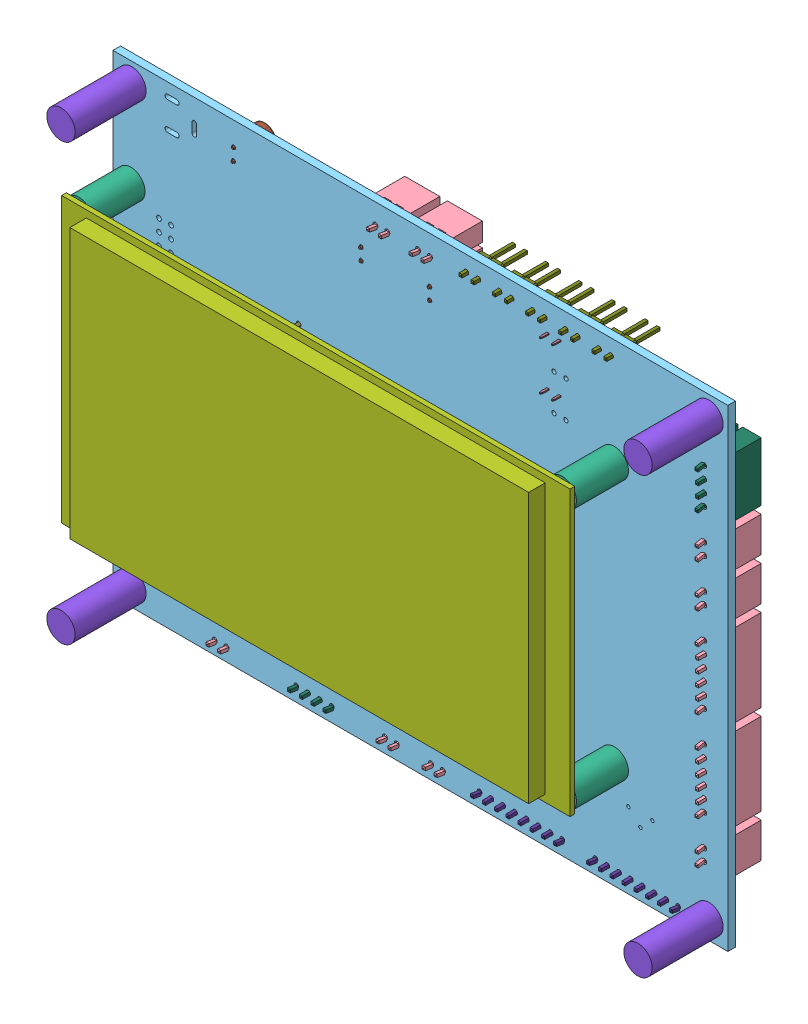
SolidWorks assembly MCU, configuration 默认. Lengths in mm.
Overall size (130 100 25.69).
427 component instances, 26 part files, 12 mates.
Components (placement in the parent):
- MCU(2)^MCU-1: MCU(2)^MCU [默认] at origin size (130 100 11.94) (virtual)
  - D_SOD-123^MCU(2)_MCU-1: D_SOD-123^MCU(2)_MCU [默认] at (95.25 63.25 -0.05) x (-1 0 0) z (0 0 -1) size (3.8 1.6 1.25) (virtual)
    - SOLID^D_SOD-123_MCU(2)_MCU-1: SOLID^D_SOD-123_MCU(2)_MCU [默认] at origin size (3.8 1.6 1.25) (virtual)
  - SOIC-8-1EP_3.9x4.9mm_P1.27mm_EP2.35x2.35mm^MCU(2)_MCU-1: SOIC-8-1EP_3.9x4.9mm_P1.27mm_EP2.35x2.35mm^MCU(2)_MCU [默认] at (12.975 8.365 -0.05) x (0 -1 0) z (0 0 -1) size (6 4.9 1.75) (virtual)
    - SOLID-0^SOIC-8-1EP_3.9x4.9mm_P1.27mm_EP2.35x2.35mm_MCU(2)_MCU-1: SOLID-0^SOIC-8-1EP_3.9x4.9mm_P1.27mm_EP2.35x2.35mm_MCU(2)_MCU [默认] at origin size (6 4.9 1.75) (virtual)
  - R_0805^MCU(2)_MCU-1: R_0805^MCU(2)_MCU [默认] at (13 3.75 -0.05) x (1 0 0) z (0 0 -1) size (2 1.25 0.5) (virtual)
    - SOLID-1^R_0805_MCU(2)_MCU-1: SOLID-1^R_0805_MCU(2)_MCU [默认] at origin size (2 1.25 0.5) (virtual)
  - R_0805^MCU(2)_MCU-2: R_0805^MCU(2)_MCU [默认] at (16.75 12 -0.05) x (0 1 0) z (0 0 -1) size (2 1.25 0.5) (virtual)
    - SOLID-1^R_0805_MCU(2)_MCU-1: SOLID-1^R_0805_MCU(2)_MCU [默认] at origin size (2 1.25 0.5) (virtual)
  - R_0805^MCU(2)_MCU-3: R_0805^MCU(2)_MCU [默认] at (8.75 12 -0.05) x (0 1 0) z (0 0 -1) size (2 1.25 0.5) (virtual)
    - SOLID-1^R_0805_MCU(2)_MCU-1: SOLID-1^R_0805_MCU(2)_MCU [默认] at origin size (2 1.25 0.5) (virtual)
  - JST_XH_B02B-XH-A_02x2.50mm_Straight^MCU(2)_MCU-1: JST_XH_B02B-XH-A_02x2.50mm_Straight^MCU(2)_MCU [默认] at (21.5 2.75 -0.05) x (1 0 0) z (0 0 -1) size (7.4 5.75 10.4) (virtual)
    - SOLID-2^JST_XH_B02B-XH-A_02x2.50mm_Straight_MCU(2)_MCU-1: SOLID-2^JST_XH_B02B-XH-A_02x2.50mm_Straight_MCU(2)_MCU [默认] at origin size (7.4 5.75 10.4) (virtual)
  - C_0805^MCU(2)_MCU-1: C_0805^MCU(2)_MCU [默认] at (12.75 13 -0.05) x (1 0 0) z (0 0 -1) size (2 1.25 0.78) (virtual)
    - SOLID-3^C_0805_MCU(2)_MCU-1: SOLID-3^C_0805_MCU(2)_MCU [默认] at origin size (2 1.25 0.78) (virtual)
  - R_0805^MCU(2)_MCU-4: R_0805^MCU(2)_MCU [默认] at (92.825 52.233 -0.05) x (1 0 0) z (0 0 -1) size (2 1.25 0.5) (virtual)
    - SOLID-1^R_0805_MCU(2)_MCU-1: SOLID-1^R_0805_MCU(2)_MCU [默认] at origin size (2 1.25 0.5) (virtual)
  - R_0805^MCU(2)_MCU-5: R_0805^MCU(2)_MCU [默认] at (92.8 50.2 -0.05) x (-1 0 0) z (0 0 -1) size (2 1.25 0.5) (virtual)
    - SOLID-1^R_0805_MCU(2)_MCU-1: SOLID-1^R_0805_MCU(2)_MCU [默认] at origin size (2 1.25 0.5) (virtual)
  - SOT-23^MCU(2)_MCU-1: SOT-23^MCU(2)_MCU [默认] at (89.35 52.05 -0.05) x (0 1 0) z (0 0 -1) size (2.5 3 1.2) (virtual)
    - SOLID-4^SOT-23_MCU(2)_MCU-1: SOLID-4^SOT-23_MCU(2)_MCU [默认] at origin size (2.5 3 1.2) (virtual)
  - D_SOD-123^MCU(2)_MCU-2: D_SOD-123^MCU(2)_MCU [默认] at (47.75 8.75 -0.05) x (1 0 0) z (0 0 -1) size (3.8 1.6 1.25) (virtual)
    - SOLID^D_SOD-123_MCU(2)_MCU-1: SOLID^D_SOD-123_MCU(2)_MCU [默认] at origin size (3.8 1.6 1.25) (virtual)
  - R_1206^MCU(2)_MCU-1: R_1206^MCU(2)_MCU [默认] at (46.8 77 -0.05) x (0 -1 0) z (0 0 -1) size (3.2 1.6 0.55) (virtual)
    - SOLID-5^R_1206_MCU(2)_MCU-1: SOLID-5^R_1206_MCU(2)_MCU [默认] at origin size (3.2 1.6 0.55) (virtual)
  - SOIC-14_3.9x8.7mm_P1.27mm^MCU(2)_MCU-1: SOIC-14_3.9x8.7mm_P1.27mm^MCU(2)_MCU [默认] at (113.4 28.8 -0.05) x (1 0 0) z (0 0 -1) size (6 8.7 1.75) (virtual)
    - SOLID-6^SOIC-14_3.9x8.7mm_P1.27mm_MCU(2)_MCU-1: SOLID-6^SOIC-14_3.9x8.7mm_P1.27mm_MCU(2)_MCU [默认] at origin size (6 8.7 1.75) (virtual)
  - R_0805^MCU(2)_MCU-6: R_0805^MCU(2)_MCU [默认] at (44 33.5 -0.05) x (0.707107 -0.707107 0) z (0 0 -1) size (2 1.25 0.5) (virtual)
    - SOLID-1^R_0805_MCU(2)_MCU-1: SOLID-1^R_0805_MCU(2)_MCU [默认] at origin size (2 1.25 0.5) (virtual)
  - C_0805^MCU(2)_MCU-2: C_0805^MCU(2)_MCU [默认] at (40.071 36.688 -0.05) x (0.707107 -0.707107 0) z (0 0 -1) size (2 1.25 0.78) (virtual)
    - SOLID-3^C_0805_MCU(2)_MCU-1: SOLID-3^C_0805_MCU(2)_MCU [默认] at origin size (2 1.25 0.78) (virtual)
  - C_0805^MCU(2)_MCU-3: C_0805^MCU(2)_MCU [默认] at (33.34 61.707 -0.05) x (-0.707107 0.707107 0) z (0 0 -1) size (2 1.25 0.78) (virtual)
    - SOLID-3^C_0805_MCU(2)_MCU-1: SOLID-3^C_0805_MCU(2)_MCU [默认] at origin size (2 1.25 0.78) (virtual)
  - C_0805^MCU(2)_MCU-4: C_0805^MCU(2)_MCU [默认] at (24.196 47.229 -0.05) x (-0.707107 -0.707107 0) z (0 0 -1) size (2 1.25 0.78) (virtual)
    - SOLID-3^C_0805_MCU(2)_MCU-1: SOLID-3^C_0805_MCU(2)_MCU [默认] at origin size (2 1.25 0.78) (virtual)
  - D_SOD-123^MCU(2)_MCU-3: D_SOD-123^MCU(2)_MCU [默认] at (70.932 14.59 -0.05) x (1 0 0) z (0 0 -1) size (3.8 1.6 1.25) (virtual)
    - SOLID^D_SOD-123_MCU(2)_MCU-1: SOLID^D_SOD-123_MCU(2)_MCU [默认] at origin size (3.8 1.6 1.25) (virtual)
  - R_0805^MCU(2)_MCU-7: R_0805^MCU(2)_MCU [默认] at (65.598 8.24 -0.05) x (-1 0 0) z (0 0 -1) size (2 1.25 0.5) (virtual)
    - SOLID-1^R_0805_MCU(2)_MCU-1: SOLID-1^R_0805_MCU(2)_MCU [默认] at origin size (2 1.25 0.5) (virtual)
  - R_0805^MCU(2)_MCU-8: R_0805^MCU(2)_MCU [默认] at (40.25 95 -0.05) x (0 -1 0) z (0 0 -1) size (2 1.25 0.5) (virtual)
    - SOLID-1^R_0805_MCU(2)_MCU-1: SOLID-1^R_0805_MCU(2)_MCU [默认] at origin size (2 1.25 0.5) (virtual)
  - R_0805^MCU(2)_MCU-9: R_0805^MCU(2)_MCU [默认] at (125.5 8.75 -0.05) x (1 0 0) z (0 0 -1) size (2 1.25 0.5) (virtual)
    - SOLID-1^R_0805_MCU(2)_MCU-1: SOLID-1^R_0805_MCU(2)_MCU [默认] at origin size (2 1.25 0.5) (virtual)
  - R_0805^MCU(2)_MCU-10: R_0805^MCU(2)_MCU [默认] at (102 34.25 -0.05) x (1 0 0) z (0 0 -1) size (2 1.25 0.5) (virtual)
    - SOLID-1^R_0805_MCU(2)_MCU-1: SOLID-1^R_0805_MCU(2)_MCU [默认] at origin size (2 1.25 0.5) (virtual)
  - R_0805^MCU(2)_MCU-11: R_0805^MCU(2)_MCU [默认] at (101.5 45.25 -0.05) x (1 0 0) z (0 0 -1) size (2 1.25 0.5) (virtual)
    - SOLID-1^R_0805_MCU(2)_MCU-1: SOLID-1^R_0805_MCU(2)_MCU [默认] at origin size (2 1.25 0.5) (virtual)
  - R_0805^MCU(2)_MCU-12: R_0805^MCU(2)_MCU [默认] at (99 73.75 -0.05) x (0 1 0) z (0 0 -1) size (2 1.25 0.5) (virtual)
    - SOLID-1^R_0805_MCU(2)_MCU-1: SOLID-1^R_0805_MCU(2)_MCU [默认] at origin size (2 1.25 0.5) (virtual)
  - R_0805^MCU(2)_MCU-13: R_0805^MCU(2)_MCU [默认] at (93.5 73.75 -0.05) x (0 1 0) z (0 0 -1) size (2 1.25 0.5) (virtual)
    - SOLID-1^R_0805_MCU(2)_MCU-1: SOLID-1^R_0805_MCU(2)_MCU [默认] at origin size (2 1.25 0.5) (virtual)
  - R_0805^MCU(2)_MCU-14: R_0805^MCU(2)_MCU [默认] at (107.5 54.75 -0.05) x (1 0 0) z (0 0 -1) size (2 1.25 0.5) (virtual)
    - SOLID-1^R_0805_MCU(2)_MCU-1: SOLID-1^R_0805_MCU(2)_MCU [默认] at origin size (2 1.25 0.5) (virtual)
  - R_0805^MCU(2)_MCU-15: R_0805^MCU(2)_MCU [默认] at (109 60.25 -0.05) x (1 0 0) z (0 0 -1) size (2 1.25 0.5) (virtual)
    - SOLID-1^R_0805_MCU(2)_MCU-1: SOLID-1^R_0805_MCU(2)_MCU [默认] at origin size (2 1.25 0.5) (virtual)
  - R_0805^MCU(2)_MCU-16: R_0805^MCU(2)_MCU [默认] at (43.25 8.45 -0.05) x (-1 0 0) z (0 0 -1) size (2 1.25 0.5) (virtual)
    - SOLID-1^R_0805_MCU(2)_MCU-1: SOLID-1^R_0805_MCU(2)_MCU [默认] at origin size (2 1.25 0.5) (virtual)
  - R_0805^MCU(2)_MCU-17: R_0805^MCU(2)_MCU [默认] at (40 8.45 -0.05) x (-1 0 0) z (0 0 -1) size (2 1.25 0.5) (virtual)
    - SOLID-1^R_0805_MCU(2)_MCU-1: SOLID-1^R_0805_MCU(2)_MCU [默认] at origin size (2 1.25 0.5) (virtual)
  - R_0805^MCU(2)_MCU-18: R_0805^MCU(2)_MCU [默认] at (83 93.5 -0.05) x (-1 0 0) z (0 0 -1) size (2 1.25 0.5) (virtual)
    - SOLID-1^R_0805_MCU(2)_MCU-1: SOLID-1^R_0805_MCU(2)_MCU [默认] at origin size (2 1.25 0.5) (virtual)
  - R_0805^MCU(2)_MCU-19: R_0805^MCU(2)_MCU [默认] at (76 93.5 -0.05) x (-1 0 0) z (0 0 -1) size (2 1.25 0.5) (virtual)
    - SOLID-1^R_0805_MCU(2)_MCU-1: SOLID-1^R_0805_MCU(2)_MCU [默认] at origin size (2 1.25 0.5) (virtual)
  - R_0805^MCU(2)_MCU-20: R_0805^MCU(2)_MCU [默认] at (90 93.5 -0.05) x (1 0 0) z (0 0 -1) size (2 1.25 0.5) (virtual)
    - SOLID-1^R_0805_MCU(2)_MCU-1: SOLID-1^R_0805_MCU(2)_MCU [默认] at origin size (2 1.25 0.5) (virtual)
  - SOIC-16_3.9x9.9mm_P1.27mm^MCU(2)_MCU-1: SOIC-16_3.9x9.9mm_P1.27mm^MCU(2)_MCU [默认] at (43.9 16.7 -0.05) x (0 -1 0) z (0 0 -1) size (6 9.9 1.75) (virtual)
    - SOLID-7^SOIC-16_3.9x9.9mm_P1.27mm_MCU(2)_MCU-1: SOLID-7^SOIC-16_3.9x9.9mm_P1.27mm_MCU(2)_MCU [默认] at origin size (6 9.9 1.75) (virtual)
  - SOT-23-5^MCU(2)_MCU-1: SOT-23-5^MCU(2)_MCU [默认] at (106.5 90 -0.05) x (-1 0 0) z (0 0 -1) size (2.8 2.9 1.55) (virtual)
    - SOLID-8^SOT-23-5_MCU(2)_MCU-1: SOLID-8^SOT-23-5_MCU(2)_MCU [默认] at origin size (2.8 2.9 1.55) (virtual)
  - R_0805^MCU(2)_MCU-21: R_0805^MCU(2)_MCU [默认] at (108.5 93.5 -0.05) x (-1 0 0) z (0 0 -1) size (2 1.25 0.5) (virtual)
    - SOLID-1^R_0805_MCU(2)_MCU-1: SOLID-1^R_0805_MCU(2)_MCU [默认] at origin size (2 1.25 0.5) (virtual)
  - C_0805^MCU(2)_MCU-5: C_0805^MCU(2)_MCU [默认] at (37.023 18.315 -0.05) x (0 1 0) z (0 0 -1) size (2 1.25 0.78) (virtual)
    - SOLID-3^C_0805_MCU(2)_MCU-1: SOLID-3^C_0805_MCU(2)_MCU [默认] at origin size (2 1.25 0.78) (virtual)
  - C_0805^MCU(2)_MCU-6: C_0805^MCU(2)_MCU [默认] at (47.765 22.2 -0.05) x (-1 0 0) z (0 0 -1) size (2 1.25 0.78) (virtual)
    - SOLID-3^C_0805_MCU(2)_MCU-1: SOLID-3^C_0805_MCU(2)_MCU [默认] at origin size (2 1.25 0.78) (virtual)
  - C_0805^MCU(2)_MCU-7: C_0805^MCU(2)_MCU [默认] at (44.015 22.2 -0.05) x (-1 0 0) z (0 0 -1) size (2 1.25 0.78) (virtual)
    - SOLID-3^C_0805_MCU(2)_MCU-1: SOLID-3^C_0805_MCU(2)_MCU [默认] at origin size (2 1.25 0.78) (virtual)
  - C_0805^MCU(2)_MCU-8: C_0805^MCU(2)_MCU [默认] at (37.15 12.812 -0.05) x (0 -1 0) z (0 0 -1) size (2 1.25 0.78) (virtual)
    - SOLID-3^C_0805_MCU(2)_MCU-1: SOLID-3^C_0805_MCU(2)_MCU [默认] at origin size (2 1.25 0.78) (virtual)
  - C_0805^MCU(2)_MCU-9: C_0805^MCU(2)_MCU [默认] at (40.265 22.2 -0.05) x (1 0 0) z (0 0 -1) size (2 1.25 0.78) (virtual)
    - SOLID-3^C_0805_MCU(2)_MCU-1: SOLID-3^C_0805_MCU(2)_MCU [默认] at origin size (2 1.25 0.78) (virtual)
  - D_SOD-123^MCU(2)_MCU-4: D_SOD-123^MCU(2)_MCU [默认] at (68.6 18.866 -0.05) x (1 0 0) z (0 0 -1) size (3.8 1.6 1.25) (virtual)
    - SOLID^D_SOD-123_MCU(2)_MCU-1: SOLID^D_SOD-123_MCU(2)_MCU [默认] at origin size (3.8 1.6 1.25) (virtual)
  - D_SOD-123^MCU(2)_MCU-5: D_SOD-123^MCU(2)_MCU [默认] at (68.6 16.866 -0.05) x (1 0 0) z (0 0 -1) size (3.8 1.6 1.25) (virtual)
    - SOLID^D_SOD-123_MCU(2)_MCU-1: SOLID^D_SOD-123_MCU(2)_MCU [默认] at origin size (3.8 1.6 1.25) (virtual)
  - SOIC-8-1EP_3.9x4.9mm_P1.27mm_EP2.35x2.35mm^MCU(2)_MCU-2: SOIC-8-1EP_3.9x4.9mm_P1.27mm_EP2.35x2.35mm^MCU(2)_MCU [默认] at (112.5 40.5 -0.05) x (0 -1 0) z (0 0 -1) size (6 4.9 1.75) (virtual)
    - SOLID-0^SOIC-8-1EP_3.9x4.9mm_P1.27mm_EP2.35x2.35mm_MCU(2)_MCU-1: SOLID-0^SOIC-8-1EP_3.9x4.9mm_P1.27mm_EP2.35x2.35mm_MCU(2)_MCU [默认] at origin size (6 4.9 1.75) (virtual)
  - R_1206^MCU(2)_MCU-2: R_1206^MCU(2)_MCU [默认] at (38.75 82.25 -0.05) x (-1 0 0) z (0 0 -1) size (3.2 1.6 0.55) (virtual)
    - SOLID-5^R_1206_MCU(2)_MCU-1: SOLID-5^R_1206_MCU(2)_MCU [默认] at origin size (3.2 1.6 0.55) (virtual)
  - R_0805^MCU(2)_MCU-22: R_0805^MCU(2)_MCU [默认] at (73 85.75 -0.05) x (0 1 0) z (0 0 -1) size (2 1.25 0.5) (virtual)
    - SOLID-1^R_0805_MCU(2)_MCU-1: SOLID-1^R_0805_MCU(2)_MCU [默认] at origin size (2 1.25 0.5) (virtual)
  - R_0805^MCU(2)_MCU-23: R_0805^MCU(2)_MCU [默认] at (71 85.75 -0.05) x (0 1 0) z (0 0 -1) size (2 1.25 0.5) (virtual)
    - SOLID-1^R_0805_MCU(2)_MCU-1: SOLID-1^R_0805_MCU(2)_MCU [默认] at origin size (2 1.25 0.5) (virtual)
  - R_0805^MCU(2)_MCU-24: R_0805^MCU(2)_MCU [默认] at (34.75 83 -0.05) x (-1 0 0) z (0 0 -1) size (2 1.25 0.5) (virtual)
    - SOLID-1^R_0805_MCU(2)_MCU-1: SOLID-1^R_0805_MCU(2)_MCU [默认] at origin size (2 1.25 0.5) (virtual)
  - R_0805^MCU(2)_MCU-25: R_0805^MCU(2)_MCU [默认] at (35.25 86 -0.05) x (0 -1 0) z (0 0 -1) size (2 1.25 0.5) (virtual)
    - SOLID-1^R_0805_MCU(2)_MCU-1: SOLID-1^R_0805_MCU(2)_MCU [默认] at origin size (2 1.25 0.5) (virtual)
  - CP_Radial_D5.0mm_P2.50mm^MCU(2)_MCU-1: CP_Radial_D5.0mm_P2.50mm^MCU(2)_MCU [默认] at (67 90.25 -0.05) x (0 -1 0) z (0 0 -1) size (6.13 6.52 7) (virtual)
    - SOLID-9^CP_Radial_D5.0mm_P2.50mm_MCU(2)_MCU-1: SOLID-9^CP_Radial_D5.0mm_P2.50mm_MCU(2)_MCU [默认] at origin size (6.13 6.52 7) (virtual)
  - C_0805^MCU(2)_MCU-10: C_0805^MCU(2)_MCU [默认] at (3.5 84 -0.05) x (0 -1 0) z (0 0 -1) size (2 1.25 0.78) (virtual)
    - SOLID-3^C_0805_MCU(2)_MCU-1: SOLID-3^C_0805_MCU(2)_MCU [默认] at origin size (2 1.25 0.78) (virtual)
  - SOIC-14_3.9x8.7mm_P1.27mm^MCU(2)_MCU-2: SOIC-14_3.9x8.7mm_P1.27mm^MCU(2)_MCU [默认] at (96.5 16.5 -0.05) x (0 -1 0) z (0 0 -1) size (6 8.7 1.75) (virtual)
    - SOLID-6^SOIC-14_3.9x8.7mm_P1.27mm_MCU(2)_MCU-1: SOLID-6^SOIC-14_3.9x8.7mm_P1.27mm_MCU(2)_MCU [默认] at origin size (6 8.7 1.75) (virtual)
  - SOIC-14_3.9x8.7mm_P1.27mm^MCU(2)_MCU-3: SOIC-14_3.9x8.7mm_P1.27mm^MCU(2)_MCU [默认] at (113.5 68 -0.05) x (1 0 0) z (0 0 -1) size (6 8.7 1.75) (virtual)
    - SOLID-6^SOIC-14_3.9x8.7mm_P1.27mm_MCU(2)_MCU-1: SOLID-6^SOIC-14_3.9x8.7mm_P1.27mm_MCU(2)_MCU [默认] at origin size (6 8.7 1.75) (virtual)
  - SOIC-14_3.9x8.7mm_P1.27mm^MCU(2)_MCU-4: SOIC-14_3.9x8.7mm_P1.27mm^MCU(2)_MCU [默认] at (113.5 52.25 -0.05) x (1 0 0) z (0 0 -1) size (6 8.7 1.75) (virtual)
    - SOLID-6^SOIC-14_3.9x8.7mm_P1.27mm_MCU(2)_MCU-1: SOLID-6^SOIC-14_3.9x8.7mm_P1.27mm_MCU(2)_MCU [默认] at origin size (6 8.7 1.75) (virtual)
  - SOIC-14_3.9x8.7mm_P1.27mm^MCU(2)_MCU-5: SOIC-14_3.9x8.7mm_P1.27mm^MCU(2)_MCU [默认] at (113.75 81.5 -0.05) x (1 0 0) z (0 0 -1) size (6 8.7 1.75) (virtual)
    - SOLID-6^SOIC-14_3.9x8.7mm_P1.27mm_MCU(2)_MCU-1: SOLID-6^SOIC-14_3.9x8.7mm_P1.27mm_MCU(2)_MCU [默认] at origin size (6 8.7 1.75) (virtual)
  - Pin_Header_Straight_1x04_Pitch2.54mm^MCU(2)_MCU-1: Pin_Header_Straight_1x04_Pitch2.54mm^MCU(2)_MCU [默认] at (44.643 64.12 -0.05) x (0.707107 0.707107 0) z (0 0 -1) size (2.54 10.16 11.54) (virtual)
    - SOLID-10^Pin_Header_Straight_1x04_Pitch2.54mm_MCU(2)_MCU-1: SOLID-10^Pin_Header_Straight_1x04_Pitch2.54mm_MCU(2)_MCU [默认] at origin size (2.54 10.16 11.54) (virtual)
  - CP_Radial_D5.0mm_P2.50mm^MCU(2)_MCU-2: CP_Radial_D5.0mm_P2.50mm^MCU(2)_MCU [默认] at (52.5 90.25 -0.05) x (0 -1 0) z (0 0 -1) size (6.13 6.52 7) (virtual)
    - SOLID-9^CP_Radial_D5.0mm_P2.50mm_MCU(2)_MCU-1: SOLID-9^CP_Radial_D5.0mm_P2.50mm_MCU(2)_MCU [默认] at origin size (6.13 6.52 7) (virtual)
  - DIP-4_W10.16mm^MCU(2)_MCU-1: DIP-4_W10.16mm^MCU(2)_MCU [默认] at (94.5 84 -0.05) x (0 1 0) z (0 0 -1) size (10.41 4.93 6.98) (virtual)
    - SOLID-11^DIP-4_W10.16mm_MCU(2)_MCU-1: SOLID-11^DIP-4_W10.16mm_MCU(2)_MCU [默认] at origin size (10.41 4.93 6.98) (virtual)
  - SOT-23-5^MCU(2)_MCU-2: SOT-23-5^MCU(2)_MCU [默认] at (61.35 18.366 -0.05) x (0 1 0) z (0 0 -1) size (2.8 2.9 1.55) (virtual)
    - SOLID-8^SOT-23-5_MCU(2)_MCU-1: SOLID-8^SOT-23-5_MCU(2)_MCU [默认] at origin size (2.8 2.9 1.55) (virtual)
  - LQFP-100_14x14mm_P0.5mm^MCU(2)_MCU-1: LQFP-100_14x14mm_P0.5mm^MCU(2)_MCU [默认] at (36.5 50 -0.05) x (-0.707107 0.707107 0) z (0 0 -1) size (16 16 1.5) (virtual)
    - SOLID-12^LQFP-100_14x14mm_P0.5mm_MCU(2)_MCU-1: SOLID-12^LQFP-100_14x14mm_P0.5mm_MCU(2)_MCU [默认] at origin size (16 16 1.5) (virtual)
  - R_0805^MCU(2)_MCU-26: R_0805^MCU(2)_MCU [默认] at (56.5 85.75 -0.05) x (0 1 0) z (0 0 -1) size (2 1.25 0.5) (virtual)
    - SOLID-1^R_0805_MCU(2)_MCU-1: SOLID-1^R_0805_MCU(2)_MCU [默认] at origin size (2 1.25 0.5) (virtual)
  - R_0805^MCU(2)_MCU-27: R_0805^MCU(2)_MCU [默认] at (58.75 84.3 -0.05) x (0 -1 0) z (0 0 -1) size (2 1.25 0.5) (virtual)
    - SOLID-1^R_0805_MCU(2)_MCU-1: SOLID-1^R_0805_MCU(2)_MCU [默认] at origin size (2 1.25 0.5) (virtual)
  - R_0805^MCU(2)_MCU-28: R_0805^MCU(2)_MCU [默认] at (31.25 83 -0.05) x (-1 0 0) z (0 0 -1) size (2 1.25 0.5) (virtual)
    - SOLID-1^R_0805_MCU(2)_MCU-1: SOLID-1^R_0805_MCU(2)_MCU [默认] at origin size (2 1.25 0.5) (virtual)
  - R_0805^MCU(2)_MCU-29: R_0805^MCU(2)_MCU [默认] at (100.75 63 -0.05) x (-1 0 0) z (0 0 -1) size (2 1.25 0.5) (virtual)
    - SOLID-1^R_0805_MCU(2)_MCU-1: SOLID-1^R_0805_MCU(2)_MCU [默认] at origin size (2 1.25 0.5) (virtual)
  - SOT-23^MCU(2)_MCU-2: SOT-23^MCU(2)_MCU [默认] at (76.25 86 -0.05) x (1 0 0) z (0 0 -1) size (2.5 3 1.2) (virtual)
    - SOLID-4^SOT-23_MCU(2)_MCU-1: SOLID-4^SOT-23_MCU(2)_MCU [默认] at origin size (2.5 3 1.2) (virtual)
  - SOT-23^MCU(2)_MCU-3: SOT-23^MCU(2)_MCU [默认] at (62 86.25 -0.05) x (1 0 0) z (0 0 -1) size (2.5 3 1.2) (virtual)
    - SOLID-4^SOT-23_MCU(2)_MCU-1: SOLID-4^SOT-23_MCU(2)_MCU [默认] at origin size (2.5 3 1.2) (virtual)
  - JST_XH_B02B-XH-A_02x2.50mm_Straight^MCU(2)_MCU-2: JST_XH_B02B-XH-A_02x2.50mm_Straight^MCU(2)_MCU [默认] at (64.5 95.75 -0.05) x (1 0 0) z (0 0 -1) size (7.4 5.75 10.4) (virtual)
    - SOLID-2^JST_XH_B02B-XH-A_02x2.50mm_Straight_MCU(2)_MCU-1: SOLID-2^JST_XH_B02B-XH-A_02x2.50mm_Straight_MCU(2)_MCU [默认] at origin size (7.4 5.75 10.4) (virtual)
  - JST_XH_B02B-XH-A_02x2.50mm_Straight^MCU(2)_MCU-3: JST_XH_B02B-XH-A_02x2.50mm_Straight^MCU(2)_MCU [默认] at (55.5 95.75 -0.05) x (1 0 0) z (0 0 -1) size (7.4 5.75 10.4) (virtual)
    - SOLID-2^JST_XH_B02B-XH-A_02x2.50mm_Straight_MCU(2)_MCU-1: SOLID-2^JST_XH_B02B-XH-A_02x2.50mm_Straight_MCU(2)_MCU [默认] at origin size (7.4 5.75 10.4) (virtual)
  - JST_XH_B04B-XH-A_04x2.50mm_Straight^MCU(2)_MCU-1: JST_XH_B04B-XH-A_04x2.50mm_Straight^MCU(2)_MCU [默认] at (38.75 3 -0.05) x (1 0 0) z (0 0 -1) size (12.4 5.75 10.4) (virtual)
    - SOLID-13^JST_XH_B04B-XH-A_04x2.50mm_Straight_MCU(2)_MCU-1: SOLID-13^JST_XH_B04B-XH-A_04x2.50mm_Straight_MCU(2)_MCU [默认] at origin size (12.4 5.75 10.4) (virtual)
  - Pin_Header_Straight_1x02_Pitch2.54mm^MCU(2)_MCU-1: Pin_Header_Straight_1x02_Pitch2.54mm^MCU(2)_MCU [默认] at (77.25 96.75 -0.05) x (0 1 0) z (0 0 -1) size (2.54 5.08 11.54) (virtual)
    - SOLID-14^Pin_Header_Straight_1x02_Pitch2.54mm_MCU(2)_MCU-1: SOLID-14^Pin_Header_Straight_1x02_Pitch2.54mm_MCU(2)_MCU [默认] at origin size (2.54 5.08 11.54) (virtual)
  - Pin_Header_Straight_1x02_Pitch2.54mm^MCU(2)_MCU-2: Pin_Header_Straight_1x02_Pitch2.54mm^MCU(2)_MCU [默认] at (95.75 96.75 -0.05) x (0 -1 0) z (0 0 -1) size (2.54 5.08 11.54) (virtual)
    - SOLID-14^Pin_Header_Straight_1x02_Pitch2.54mm_MCU(2)_MCU-1: SOLID-14^Pin_Header_Straight_1x02_Pitch2.54mm_MCU(2)_MCU [默认] at origin size (2.54 5.08 11.54) (virtual)
  - JST_XH_B02B-XH-A_02x2.50mm_Straight^MCU(2)_MCU-4: JST_XH_B02B-XH-A_02x2.50mm_Straight^MCU(2)_MCU [默认] at (57.5 3 -0.05) x (1 0 0) z (0 0 -1) size (7.4 5.75 10.4) (virtual)
    - SOLID-2^JST_XH_B02B-XH-A_02x2.50mm_Straight_MCU(2)_MCU-1: SOLID-2^JST_XH_B02B-XH-A_02x2.50mm_Straight_MCU(2)_MCU [默认] at origin size (7.4 5.75 10.4) (virtual)
  - JST_XH_B08B-XH-A_08x2.50mm_Straight^MCU(2)_MCU-1: JST_XH_B08B-XH-A_08x2.50mm_Straight^MCU(2)_MCU [默认] at (102 3 -0.05) x (1 0 0) z (0 0 -1) size (22.4 5.75 10.4) (virtual)
    - SOLID-15^JST_XH_B08B-XH-A_08x2.50mm_Straight_MCU(2)_MCU-1: SOLID-15^JST_XH_B08B-XH-A_08x2.50mm_Straight_MCU(2)_MCU [默认] at origin size (22.4 5.75 10.4) (virtual)
  - JST_XH_B08B-XH-A_08x2.50mm_Straight^MCU(2)_MCU-2: JST_XH_B08B-XH-A_08x2.50mm_Straight^MCU(2)_MCU [默认] at (77.5 3 -0.05) x (1 0 0) z (0 0 -1) size (22.4 5.75 10.4) (virtual)
    - SOLID-15^JST_XH_B08B-XH-A_08x2.50mm_Straight_MCU(2)_MCU-1: SOLID-15^JST_XH_B08B-XH-A_08x2.50mm_Straight_MCU(2)_MCU [默认] at origin size (22.4 5.75 10.4) (virtual)
  - C_0805^MCU(2)_MCU-11: C_0805^MCU(2)_MCU [默认] at (43 82.25 -0.05) x (1 0 0) z (0 0 -1) size (2 1.25 0.78) (virtual)
    - SOLID-3^C_0805_MCU(2)_MCU-1: SOLID-3^C_0805_MCU(2)_MCU [默认] at origin size (2 1.25 0.78) (virtual)
  - C_0805^MCU(2)_MCU-12: C_0805^MCU(2)_MCU [默认] at (37 90.75 -0.05) x (0 -1 0) z (0 0 -1) size (2 1.25 0.78) (virtual)
    - SOLID-3^C_0805_MCU(2)_MCU-1: SOLID-3^C_0805_MCU(2)_MCU [默认] at origin size (2 1.25 0.78) (virtual)
  - CP_Radial_D5.0mm_P2.50mm^MCU(2)_MCU-3: CP_Radial_D5.0mm_P2.50mm^MCU(2)_MCU [默认] at (25.5 92.5 -0.05) x (0 1 0) z (0 0 -1) size (6.13 6.52 7) (virtual)
    - SOLID-9^CP_Radial_D5.0mm_P2.50mm_MCU(2)_MCU-1: SOLID-9^CP_Radial_D5.0mm_P2.50mm_MCU(2)_MCU [默认] at origin size (6.13 6.52 7) (virtual)
  - SOT-223^MCU(2)_MCU-1: SOT-223^MCU(2)_MCU [默认] at (9.5 85.5 -0.05) x (1 0 0) z (0 0 -1) size (7 6.5 1.7) (virtual)
    - SOLID-16^SOT-223_MCU(2)_MCU-1: SOLID-16^SOT-223_MCU(2)_MCU [默认] at origin size (7 6.5 1.7) (virtual)
  - SOT-223^MCU(2)_MCU-2: SOT-223^MCU(2)_MCU [默认] at (41.75 88.5 -0.05) x (0 1 0) z (0 0 -1) size (7 6.5 1.7) (virtual)
    - SOLID-16^SOT-223_MCU(2)_MCU-1: SOLID-16^SOT-223_MCU(2)_MCU [默认] at origin size (7 6.5 1.7) (virtual)
  - TSOT-23-8^MCU(2)_MCU-1: TSOT-23-8^MCU(2)_MCU [默认] at (32 87.25 -0.05) x (0 1 0) z (0 0 -1) size (2.8 2.9 0.95) (virtual)
    - SOLID-17^TSOT-23-8_MCU(2)_MCU-1: SOLID-17^TSOT-23-8_MCU(2)_MCU [默认] at origin size (2.8 2.9 0.95) (virtual)
  - SOIC-8-1EP_3.9x4.9mm_P1.27mm_EP2.35x2.35mm^MCU(2)_MCU-3: SOIC-8-1EP_3.9x4.9mm_P1.27mm_EP2.35x2.35mm^MCU(2)_MCU [默认] at (100.25 89.5 -0.05) x (0 1 0) z (0 0 -1) size (6 4.9 1.75) (virtual)
    - SOLID-0^SOIC-8-1EP_3.9x4.9mm_P1.27mm_EP2.35x2.35mm_MCU(2)_MCU-1: SOLID-0^SOIC-8-1EP_3.9x4.9mm_P1.27mm_EP2.35x2.35mm_MCU(2)_MCU [默认] at origin size (6 4.9 1.75) (virtual)
  - SOT-23-5^MCU(2)_MCU-3: SOT-23-5^MCU(2)_MCU [默认] at (119.4 14.3 -0.05) x (-1 0 0) z (0 0 -1) size (2.8 2.9 1.55) (virtual)
    - SOLID-8^SOT-23-5_MCU(2)_MCU-1: SOLID-8^SOT-23-5_MCU(2)_MCU [默认] at origin size (2.8 2.9 1.55) (virtual)
  - R_0805^MCU(2)_MCU-30: R_0805^MCU(2)_MCU [默认] at (26 88.5 -0.05) x (0 -1 0) z (0 0 -1) size (2 1.25 0.5) (virtual)
    - SOLID-1^R_0805_MCU(2)_MCU-1: SOLID-1^R_0805_MCU(2)_MCU [默认] at origin size (2 1.25 0.5) (virtual)
  - R_0805^MCU(2)_MCU-31: R_0805^MCU(2)_MCU [默认] at (105 93.5 -0.05) x (1 0 0) z (0 0 -1) size (2 1.25 0.5) (virtual)
    - SOLID-1^R_0805_MCU(2)_MCU-1: SOLID-1^R_0805_MCU(2)_MCU [默认] at origin size (2 1.25 0.5) (virtual)
  - R_0805^MCU(2)_MCU-32: R_0805^MCU(2)_MCU [默认] at (52.65 10.95 -0.05) x (1 0 0) z (0 0 -1) size (2 1.25 0.5) (virtual)
    - SOLID-1^R_0805_MCU(2)_MCU-1: SOLID-1^R_0805_MCU(2)_MCU [默认] at origin size (2 1.25 0.5) (virtual)
  - R_0805^MCU(2)_MCU-33: R_0805^MCU(2)_MCU [默认] at (52.65 12.95 -0.05) x (1 0 0) z (0 0 -1) size (2 1.25 0.5) (virtual)
    - SOLID-1^R_0805_MCU(2)_MCU-1: SOLID-1^R_0805_MCU(2)_MCU [默认] at origin size (2 1.25 0.5) (virtual)
  - R_0805^MCU(2)_MCU-34: R_0805^MCU(2)_MCU [默认] at (100.45 59.25 -0.05) x (-1 0 0) z (0 0 -1) size (2 1.25 0.5) (virtual)
    - SOLID-1^R_0805_MCU(2)_MCU-1: SOLID-1^R_0805_MCU(2)_MCU [默认] at origin size (2 1.25 0.5) (virtual)
  - R_0805^MCU(2)_MCU-35: R_0805^MCU(2)_MCU [默认] at (96.25 54.5 -0.05) x (-1 0 0) z (0 0 -1) size (2 1.25 0.5) (virtual)
    - SOLID-1^R_0805_MCU(2)_MCU-1: SOLID-1^R_0805_MCU(2)_MCU [默认] at origin size (2 1.25 0.5) (virtual)
  - R_0805^MCU(2)_MCU-36: R_0805^MCU(2)_MCU [默认] at (99.75 50.25 -0.05) x (1 0 0) z (0 0 -1) size (2 1.25 0.5) (virtual)
    - SOLID-1^R_0805_MCU(2)_MCU-1: SOLID-1^R_0805_MCU(2)_MCU [默认] at origin size (2 1.25 0.5) (virtual)
  - R_0805^MCU(2)_MCU-37: R_0805^MCU(2)_MCU [默认] at (92.65 54.4 -0.05) x (1 0 0) z (0 0 -1) size (2 1.25 0.5) (virtual)
    - SOLID-1^R_0805_MCU(2)_MCU-1: SOLID-1^R_0805_MCU(2)_MCU [默认] at origin size (2 1.25 0.5) (virtual)
  - R_0805^MCU(2)_MCU-38: R_0805^MCU(2)_MCU [默认] at (92.903 47.991 -0.05) x (-1 0 0) z (0 0 -1) size (2 1.25 0.5) (virtual)
    - SOLID-1^R_0805_MCU(2)_MCU-1: SOLID-1^R_0805_MCU(2)_MCU [默认] at origin size (2 1.25 0.5) (virtual)
  - R_0805^MCU(2)_MCU-39: R_0805^MCU(2)_MCU [默认] at (87.5 85.5 -0.05) x (0 -1 0) z (0 0 -1) size (2 1.25 0.5) (virtual)
    - SOLID-1^R_0805_MCU(2)_MCU-1: SOLID-1^R_0805_MCU(2)_MCU [默认] at origin size (2 1.25 0.5) (virtual)
  - R_0805^MCU(2)_MCU-40: R_0805^MCU(2)_MCU [默认] at (67.35 27.866 -0.05) x (-1 0 0) z (0 0 -1) size (2 1.25 0.5) (virtual)
    - SOLID-1^R_0805_MCU(2)_MCU-1: SOLID-1^R_0805_MCU(2)_MCU [默认] at origin size (2 1.25 0.5) (virtual)
  - R_0805^MCU(2)_MCU-41: R_0805^MCU(2)_MCU [默认] at (64.6 25.116 -0.05) x (0 1 0) z (0 0 -1) size (2 1.25 0.5) (virtual)
    - SOLID-1^R_0805_MCU(2)_MCU-1: SOLID-1^R_0805_MCU(2)_MCU [默认] at origin size (2 1.25 0.5) (virtual)
  - R_0805^MCU(2)_MCU-42: R_0805^MCU(2)_MCU [默认] at (90.75 81.5 -0.05) x (0 1 0) z (0 0 -1) size (2 1.25 0.5) (virtual)
    - SOLID-1^R_0805_MCU(2)_MCU-1: SOLID-1^R_0805_MCU(2)_MCU [默认] at origin size (2 1.25 0.5) (virtual)
  - R_0805^MCU(2)_MCU-43: R_0805^MCU(2)_MCU [默认] at (69.4 12.149 -0.05) x (-1 0 0) z (0 0 -1) size (2 1.25 0.5) (virtual)
    - SOLID-1^R_0805_MCU(2)_MCU-1: SOLID-1^R_0805_MCU(2)_MCU [默认] at origin size (2 1.25 0.5) (virtual)
  - R_0805^MCU(2)_MCU-44: R_0805^MCU(2)_MCU [默认] at (67.35 21.366 -0.05) x (1 0 0) z (0 0 -1) size (2 1.25 0.5) (virtual)
    - SOLID-1^R_0805_MCU(2)_MCU-1: SOLID-1^R_0805_MCU(2)_MCU [默认] at origin size (2 1.25 0.5) (virtual)
  - R_0805^MCU(2)_MCU-45: R_0805^MCU(2)_MCU [默认] at (58.35 14.35 -0.05) x (0 -1 0) z (0 0 -1) size (2 1.25 0.5) (virtual)
    - SOLID-1^R_0805_MCU(2)_MCU-1: SOLID-1^R_0805_MCU(2)_MCU [默认] at origin size (2 1.25 0.5) (virtual)
  - R_0805^MCU(2)_MCU-46: R_0805^MCU(2)_MCU [默认] at (64.35 18.366 -0.05) x (0 1 0) z (0 0 -1) size (2 1.25 0.5) (virtual)
    - SOLID-1^R_0805_MCU(2)_MCU-1: SOLID-1^R_0805_MCU(2)_MCU [默认] at origin size (2 1.25 0.5) (virtual)
  - R_0805^MCU(2)_MCU-47: R_0805^MCU(2)_MCU [默认] at (94.25 91 -0.05) x (0 -1 0) z (0 0 -1) size (2 1.25 0.5) (virtual)
    - SOLID-1^R_0805_MCU(2)_MCU-1: SOLID-1^R_0805_MCU(2)_MCU [默认] at origin size (2 1.25 0.5) (virtual)
  - R_0805^MCU(2)_MCU-48: R_0805^MCU(2)_MCU [默认] at (66.614 13.447 -0.05) x (0 -1 0) z (0 0 -1) size (2 1.25 0.5) (virtual)
    - SOLID-1^R_0805_MCU(2)_MCU-1: SOLID-1^R_0805_MCU(2)_MCU [默认] at origin size (2 1.25 0.5) (virtual)
  - R_0805^MCU(2)_MCU-49: R_0805^MCU(2)_MCU [默认] at (58.35 18.866 -0.05) x (0 -1 0) z (0 0 -1) size (2 1.25 0.5) (virtual)
    - SOLID-1^R_0805_MCU(2)_MCU-1: SOLID-1^R_0805_MCU(2)_MCU [默认] at origin size (2 1.25 0.5) (virtual)
  - R_0805^MCU(2)_MCU-50: R_0805^MCU(2)_MCU [默认] at (120 17.5 -0.05) x (-1 0 0) z (0 0 -1) size (2 1.25 0.5) (virtual)
    - SOLID-1^R_0805_MCU(2)_MCU-1: SOLID-1^R_0805_MCU(2)_MCU [默认] at origin size (2 1.25 0.5) (virtual)
  - R_0805^MCU(2)_MCU-51: R_0805^MCU(2)_MCU [默认] at (120 19.5 -0.05) x (-1 0 0) z (0 0 -1) size (2 1.25 0.5) (virtual)
    - SOLID-1^R_0805_MCU(2)_MCU-1: SOLID-1^R_0805_MCU(2)_MCU [默认] at origin size (2 1.25 0.5) (virtual)
  - R_0805^MCU(2)_MCU-52: R_0805^MCU(2)_MCU [默认] at (120 75 -0.05) x (-1 0 0) z (0 0 -1) size (2 1.25 0.5) (virtual)
    - SOLID-1^R_0805_MCU(2)_MCU-1: SOLID-1^R_0805_MCU(2)_MCU [默认] at origin size (2 1.25 0.5) (virtual)
  - R_0805^MCU(2)_MCU-53: R_0805^MCU(2)_MCU [默认] at (120 65 -0.05) x (-1 0 0) z (0 0 -1) size (2 1.25 0.5) (virtual)
    - SOLID-1^R_0805_MCU(2)_MCU-1: SOLID-1^R_0805_MCU(2)_MCU [默认] at origin size (2 1.25 0.5) (virtual)
  - R_0805^MCU(2)_MCU-54: R_0805^MCU(2)_MCU [默认] at (120 53 -0.05) x (-1 0 0) z (0 0 -1) size (2 1.25 0.5) (virtual)
    - SOLID-1^R_0805_MCU(2)_MCU-1: SOLID-1^R_0805_MCU(2)_MCU [默认] at origin size (2 1.25 0.5) (virtual)
  - R_0805^MCU(2)_MCU-55: R_0805^MCU(2)_MCU [默认] at (120 49 -0.05) x (1 0 0) z (0 0 -1) size (2 1.25 0.5) (virtual)
    - SOLID-1^R_0805_MCU(2)_MCU-1: SOLID-1^R_0805_MCU(2)_MCU [默认] at origin size (2 1.25 0.5) (virtual)
  - R_0805^MCU(2)_MCU-56: R_0805^MCU(2)_MCU [默认] at (120 45 -0.05) x (-1 0 0) z (0 0 -1) size (2 1.25 0.5) (virtual)
    - SOLID-1^R_0805_MCU(2)_MCU-1: SOLID-1^R_0805_MCU(2)_MCU [默认] at origin size (2 1.25 0.5) (virtual)
  - R_0805^MCU(2)_MCU-57: R_0805^MCU(2)_MCU [默认] at (120 41 -0.05) x (-1 0 0) z (0 0 -1) size (2 1.25 0.5) (virtual)
    - SOLID-1^R_0805_MCU(2)_MCU-1: SOLID-1^R_0805_MCU(2)_MCU [默认] at origin size (2 1.25 0.5) (virtual)
  - R_0805^MCU(2)_MCU-58: R_0805^MCU(2)_MCU [默认] at (120 34.5 -0.05) x (-1 0 0) z (0 0 -1) size (2 1.25 0.5) (virtual)
    - SOLID-1^R_0805_MCU(2)_MCU-1: SOLID-1^R_0805_MCU(2)_MCU [默认] at origin size (2 1.25 0.5) (virtual)
  - R_0805^MCU(2)_MCU-59: R_0805^MCU(2)_MCU [默认] at (120 30.5 -0.05) x (-1 0 0) z (0 0 -1) size (2 1.25 0.5) (virtual)
    - SOLID-1^R_0805_MCU(2)_MCU-1: SOLID-1^R_0805_MCU(2)_MCU [默认] at origin size (2 1.25 0.5) (virtual)
  - R_0805^MCU(2)_MCU-60: R_0805^MCU(2)_MCU [默认] at (120 26.5 -0.05) x (-1 0 0) z (0 0 -1) size (2 1.25 0.5) (virtual)
    - SOLID-1^R_0805_MCU(2)_MCU-1: SOLID-1^R_0805_MCU(2)_MCU [默认] at origin size (2 1.25 0.5) (virtual)
  - R_0805^MCU(2)_MCU-61: R_0805^MCU(2)_MCU [默认] at (120 22.5 -0.05) x (-1 0 0) z (0 0 -1) size (2 1.25 0.5) (virtual)
    - SOLID-1^R_0805_MCU(2)_MCU-1: SOLID-1^R_0805_MCU(2)_MCU [默认] at origin size (2 1.25 0.5) (virtual)
  - R_0805^MCU(2)_MCU-62: R_0805^MCU(2)_MCU [默认] at (114 35.75 -0.05) x (-1 0 0) z (0 0 -1) size (2 1.25 0.5) (virtual)
    - SOLID-1^R_0805_MCU(2)_MCU-1: SOLID-1^R_0805_MCU(2)_MCU [默认] at origin size (2 1.25 0.5) (virtual)
  - R_0805^MCU(2)_MCU-63: R_0805^MCU(2)_MCU [默认] at (109.4 35.65 -0.05) x (-1 0 0) z (0 0 -1) size (2 1.25 0.5) (virtual)
    - SOLID-1^R_0805_MCU(2)_MCU-1: SOLID-1^R_0805_MCU(2)_MCU [默认] at origin size (2 1.25 0.5) (virtual)
  - R_0805^MCU(2)_MCU-64: R_0805^MCU(2)_MCU [默认] at (112.75 45.25 -0.05) x (-1 0 0) z (0 0 -1) size (2 1.25 0.5) (virtual)
    - SOLID-1^R_0805_MCU(2)_MCU-1: SOLID-1^R_0805_MCU(2)_MCU [默认] at origin size (2 1.25 0.5) (virtual)
  - R_0805^MCU(2)_MCU-65: R_0805^MCU(2)_MCU [默认] at (108.5 42.5 -0.05) x (0 -1 0) z (0 0 -1) size (2 1.25 0.5) (virtual)
    - SOLID-1^R_0805_MCU(2)_MCU-1: SOLID-1^R_0805_MCU(2)_MCU [默认] at origin size (2 1.25 0.5) (virtual)
  - R_0805^MCU(2)_MCU-66: R_0805^MCU(2)_MCU [默认] at (120 71 -0.05) x (-1 0 0) z (0 0 -1) size (2 1.25 0.5) (virtual)
    - SOLID-1^R_0805_MCU(2)_MCU-1: SOLID-1^R_0805_MCU(2)_MCU [默认] at origin size (2 1.25 0.5) (virtual)
  - R_0805^MCU(2)_MCU-67: R_0805^MCU(2)_MCU [默认] at (119.5 67 -0.05) x (-1 0 0) z (0 0 -1) size (2 1.25 0.5) (virtual)
    - SOLID-1^R_0805_MCU(2)_MCU-1: SOLID-1^R_0805_MCU(2)_MCU [默认] at origin size (2 1.25 0.5) (virtual)
  - R_0805^MCU(2)_MCU-68: R_0805^MCU(2)_MCU [默认] at (113.5 62.1 -0.05) x (-1 0 0) z (0 0 -1) size (2 1.25 0.5) (virtual)
    - SOLID-1^R_0805_MCU(2)_MCU-1: SOLID-1^R_0805_MCU(2)_MCU [默认] at origin size (2 1.25 0.5) (virtual)
  - R_0805^MCU(2)_MCU-69: R_0805^MCU(2)_MCU [默认] at (120 61 -0.05) x (-1 0 0) z (0 0 -1) size (2 1.25 0.5) (virtual)
    - SOLID-1^R_0805_MCU(2)_MCU-1: SOLID-1^R_0805_MCU(2)_MCU [默认] at origin size (2 1.25 0.5) (virtual)
  - R_0805^MCU(2)_MCU-70: R_0805^MCU(2)_MCU [默认] at (106.5 69.6 -0.05) x (1 0 0) z (0 0 -1) size (2 1.25 0.5) (virtual)
    - SOLID-1^R_0805_MCU(2)_MCU-1: SOLID-1^R_0805_MCU(2)_MCU [默认] at origin size (2 1.25 0.5) (virtual)
  - R_0805^MCU(2)_MCU-71: R_0805^MCU(2)_MCU [默认] at (106.5 67.6 -0.05) x (1 0 0) z (0 0 -1) size (2 1.25 0.5) (virtual)
    - SOLID-1^R_0805_MCU(2)_MCU-1: SOLID-1^R_0805_MCU(2)_MCU [默认] at origin size (2 1.25 0.5) (virtual)
  - R_0805^MCU(2)_MCU-72: R_0805^MCU(2)_MCU [默认] at (119.5 79 -0.05) x (-1 0 0) z (0 0 -1) size (2 1.25 0.5) (virtual)
    - SOLID-1^R_0805_MCU(2)_MCU-1: SOLID-1^R_0805_MCU(2)_MCU [默认] at origin size (2 1.25 0.5) (virtual)
  - R_0805^MCU(2)_MCU-73: R_0805^MCU(2)_MCU [默认] at (114.25 75.5 -0.05) x (-1 0 0) z (0 0 -1) size (2 1.25 0.5) (virtual)
    - SOLID-1^R_0805_MCU(2)_MCU-1: SOLID-1^R_0805_MCU(2)_MCU [默认] at origin size (2 1.25 0.5) (virtual)
  - R_0805^MCU(2)_MCU-74: R_0805^MCU(2)_MCU [默认] at (120 82.5 -0.05) x (-1 0 0) z (0 0 -1) size (2 1.25 0.5) (virtual)
    - SOLID-1^R_0805_MCU(2)_MCU-1: SOLID-1^R_0805_MCU(2)_MCU [默认] at origin size (2 1.25 0.5) (virtual)
  - R_0805^MCU(2)_MCU-75: R_0805^MCU(2)_MCU [默认] at (107.6 86.5 -0.05) x (1 0 0) z (0 0 -1) size (2 1.25 0.5) (virtual)
    - SOLID-1^R_0805_MCU(2)_MCU-1: SOLID-1^R_0805_MCU(2)_MCU [默认] at origin size (2 1.25 0.5) (virtual)
